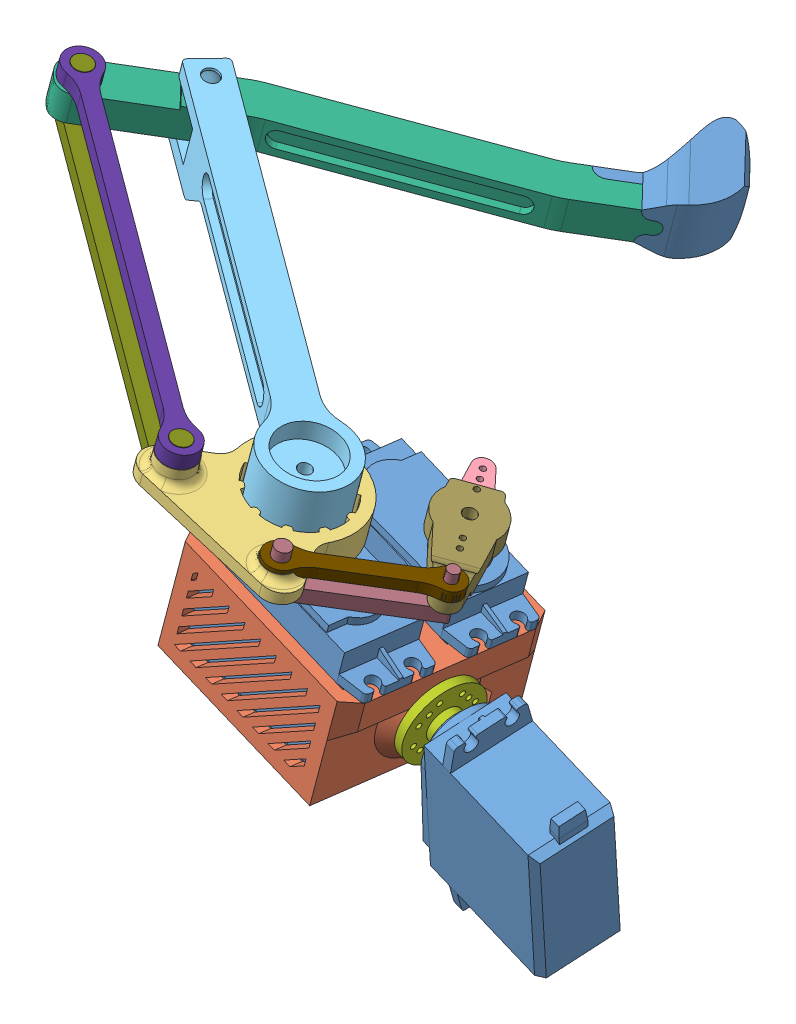
SolidWorks assembly Leg 3, configuration Default. Lengths in mm.
Overall size (184.01 129.02 174.38).
32 component instances, 19 part files, 45 mates.
Components (placement in the parent):
- MG996R-1: MG996R [Default] at (29.5952 -122.5628 58.2658) x (-0.962615 0.249609 -0.105199) z (0.100626 -0.031047 -0.99444) size (54.5 42.75 20)
- MG996R-2: MG996R [Default] at (26.9789 -121.7556 84.1213) x (0.962615 -0.249609 0.105199) z (-0.100626 0.031047 0.99444) size (54.5 42.75 20)
- MG996R-3: MG996R [Default] at (99.0906 -137.4824 76.1232) x (-0.215615 -0.941176 -0.26019) z (0.163956 0.22778 -0.95981) size (54.5 42.75 20)
- Servo Housing-1: Servo Housing [Default] at (37.077 -93.7693 58.1239) x (-0.962615 0.249609 -0.105199) z (0.251487 0.967849 -0.00477) size (61.5 52 29.25)
- Rotating Piece-1: Rotating Piece [Default] at (26.8579 -80.6595 82.9278) x (0.330954 -0.090624 -0.939285) z (0.909518 -0.23464 0.343104) size (44.28 13.7 43.21)
- Double_Blade_Rudder-1: Double_Blade_Rudder [默认] at (51.0424 -81.5852 59.0548) x (0.795547 -0.209518 -0.568514) z (-0.551235 0.13918 -0.82266) size (12.2 5.5 38)
- Upper Leg-1: Upper Leg [Default] at (-58.7777 -49.0599 29.9672) x (-0.525433 0.140664 0.839127) z (0.251487 0.967849 -0.00477) size (22 116.4 18)
- Lower leg-1: Lower leg [Default] at (27.9487 -66.2146 -31.3691) x (0.681118 -0.173478 0.711325) z (-0.251487 -0.967849 0.00477) size (20.21 126 9.59)
- Circle Rudder-1: Circle Rudder [默认] at (57.8128 -116.2822 73.9977) x (0.107242 0.707834 0.698191) z (0.248738 0.660808 -0.70814) size (20.8 5.5 20.8)
- 688ZZ Bearing Assembly-2: 688ZZ Bearing Assembly [Default] at (1.0185 -101.5553 67.791) x (-0.264501 -0.949925 0.166376) z (-0.962615 0.249609 -0.105199) size (17.99 17.98 5)
  - Outer Ring-1: Outer Ring [Default] at origin size (16 16 5)
  - Inner Ring-1: Inner Ring [Default] x (-0.241565 -0.970385 0) z (0 0 1) size (10.6 10.6 5)
  - Cage-1: Cage [Default] x (0.535517 0.844524 0) z (0 0 1) size (13.01 13.06 2.21)
  - 2mm Ball Bearing-1: 2mm Ball Bearing [Default] at (-5.0671 3.2131 0) x (0.050652 0.835774 0.546732) z (0.977207 -0.154478 0.145614) size (2 2 2)
  - 2mm Ball Bearing-2: 2mm Ball Bearing [Default] at (-5.988 -0.3789 0) x (-0.450278 0.705928 0.546732) z (0.881377 0.449412 0.145614) size (2 2 2)
  - 2mm Ball Bearing-3: 2mm Ball Bearing [Default] at (-4.6217 -3.8262 0) x (-0.779216 0.306441 0.546732) z (0.448891 0.881642 0.145614) size (2 2 2)
  - 2mm Ball Bearing-4: 2mm Ball Bearing [Default] at (-1.49 -5.812 0) x (-0.810521 -0.210096 0.546732) z (-0.155056 0.977115 0.145614) size (2 2 2)
  - 2mm Ball Bearing-5: 2mm Ball Bearing [Default] at (2.2108 -5.5778 0) x (-0.532234 -0.646383 0.546732) z (-0.699777 0.699363 0.145614) size (2 2 2)
  - 2mm Ball Bearing-6: 2mm Ball Bearing [Default] at (5.0671 -3.2131 0) x (-0.050652 -0.835774 0.546732) z (-0.977207 0.154478 0.145614) size (2 2 2)
  - 2mm Ball Bearing-7: 2mm Ball Bearing [Default] at (5.988 0.3789 0) x (0.450278 -0.705928 0.546732) z (-0.881377 -0.449412 0.145614) size (2 2 2)
  - 2mm Ball Bearing-8: 2mm Ball Bearing [Default] at (4.6217 3.8262 0) x (0.779216 -0.306441 0.546732) z (-0.448891 -0.881642 0.145614) size (2 2 2)
  - 2mm Ball Bearing-9: 2mm Ball Bearing [Default] at (1.49 5.812 0) x (0.810521 0.210096 0.546732) z (0.155056 -0.977115 0.145614) size (2 2 2)
  - 2mm Ball Bearing-10: 2mm Ball Bearing [Default] at (-2.2108 5.5778 0) x (0.532234 0.646383 0.546732) z (0.699777 -0.699363 0.145614) size (2 2 2)
- Circle Rudder-3: Circle Rudder [默认] at (28.1908 -75.5299 82.9026) x (0.821577 -0.21087 0.529666) z (0.511631 -0.137123 -0.848193) size (20.8 5.5 20.8)
- Servo Arm Mount-1: Servo Arm Mount [Default] at (51.0424 -81.5852 59.0548) x (-0.795547 0.209518 0.568514) z (0.251487 0.967849 -0.00477) size (16.2 34.39 10.1)
- Short Connecting Rod-1: Short Connecting Rod [Default] at (63.2593 -84.1638 75.1548) x (-0.680525 0.180329 0.710188) z (-0.251487 -0.967849 0.00477) size (37.08 6.33 13)
- 91595A167_Dowel Pin-1: 91595A167_Dowel Pin [91595A167] at (-52.4141 -50.7218 28.2719) x (-0.945505 0.244623 -0.214897) z (-0.251487 -0.967849 0.00477) size (4 4 20)
- Rod Cap-2: Rod Cap [Default] at (14.1029 -69.8044 103.5679) x (-0.058992 0.020247 0.998053) z (0.966061 -0.250717 0.062188) size (6.08 7 3)
- Long Connecting Rod-1: Long Connecting Rod [Default] at (14.4682 -71.3647 99.7299) x (0.812824 -0.208525 0.543906) z (-0.251487 -0.967849 0.00477) size (105.4 5 16.7)
- Long Connecting Rod Alt-1: Long Connecting Rod Alt [Default] at (13.1093 -62.8457 100.4303) x (0.812824 -0.208525 0.543906) z (-0.525424 0.140662 0.839132) size (109.5 4 9.1)
- Short Connecting Rod Alt-1: Short Connecting Rod Alt [Default] at (41.5823 -75.0354 101.4606) x (-0.680525 0.180329 0.710188) z (-0.688214 0.175358 -0.703996) size (41.18 3 8.1)
- Foot Cap R2-1: Foot Cap R2 [Default] at (27.9487 -66.2146 -31.3691) x (0.681118 -0.173478 0.711325) z (-0.251487 -0.967849 0.00477) size (26.22 31.5 15)
Mates (geometry in assembly coordinates):
- Coincident3: coincident aligned: plane of MG996R-1 through (49.2065 -88.6505 59.0896) normal (0.251487 0.967849 -0.00477); plane of MG996R-2 through (26.3549 -82.5952 82.9374) normal (0.251487 0.967849 -0.00477)
- Coincident4: coincident aligned: plane of MG996R-1 through (59.0851 -93.3273 50.2812) normal (0.962615 -0.249609 0.105199); plane of MG996R-2 through (54.4563 -91.8991 96.0254) normal (0.962615 -0.249609 0.105199)
- Distance1: distance = 6 mm anti-aligned: plane of MG996R-1 through (57.0726 -92.7063 70.17) normal (-0.100626 0.031047 0.99444); plane of MG996R-2 through (17.4829 -82.4109 71.8761) normal (0.100626 -0.031047 -0.99444)
- InPlace1: in place: plane of ? through (-38.4551 28.1284 17.4765) normal (0 1 0); plane of ? through (0 28.1284 0) normal (0 1 0); moOrthogonalPlaneRef_w of ? through (-38.4551 28.1284 17.4765) normal (0 1 0); plane of ? through (0 28.1284 0) normal (0 0 -1); plane of ? through (-38.4551 28.1284 17.4765) normal (0 1 0); plane of ? through (0 28.1284 0) normal (1 0 0); plane of MG996R-1 through (12.5314 -87.3809 60.2393) normal (0.251487 0.967849 -0.00477); unknown of Servo Housing-1
- Coincident6: coincident aligned: plane of MG996R-1; plane of Servo Housing-1
- Coincident7: coincident aligned: moOrthogonalPlaneRef_w of MG996R-1; plane of Servo Housing-1 through (37.077 -93.7693 58.1239) normal (-0.100626 0.031047 0.99444)
- Coincident8: coincident anti-aligned: moOrthogonalPlaneRef_w of MG996R-1; plane of Servo Housing-1 through (37.077 -93.7693 58.1239) normal (-0.962615 0.249609 -0.105199)
- Concentric4: concentric aligned: cylinder of Upper Leg-1 through (-54.426 -58.4646 28.3101) axis (0.251487 0.967849 -0.00477) radius 2.1; cylinder of Lower leg-1 through (-53.2943 -54.1092 28.2886) axis (0.251487 0.967849 -0.00477) radius 2
- LimitAngle3: limit planar angle = 1.561857 rad anti-aligned: plane of Lower leg-1 through (25.6853 -74.9252 -31.3262) normal (0.681118 -0.173478 0.711325); plane of Upper Leg-1 through (-51.0085 -40.788 21.5283) normal (0.525433 -0.140664 -0.839127)
- Coincident17: coincident anti-aligned: plane of Servo Housing-1 through (36.8825 -202.2704 61.4918) normal (0.962615 -0.249609 0.105199); plane of Circle Rudder-1 through (57.8128 -116.2822 73.9977) normal (-0.962615 0.249609 -0.105199)
- Concentric10: concentric aligned: circle of Servo Housing-1; circle of Circle Rudder-1
- Concentric11: concentric anti-aligned: cylinder of Servo Housing-1 through (-1.388 -100.9312 67.528) axis (0.962615 -0.249609 0.105199) radius 4; cylinder of 688ZZ Bearing Assembly-2/Inner Ring-1 through (-5.4843 -99.8691 67.0803) axis (-0.962615 0.249609 -0.105199) radius 4
- Coincident18: coincident aligned: plane of Servo Housing-1 through (4.1074 -85.2202 54.5209) normal (-0.962615 0.249609 -0.105199); plane of 688ZZ Bearing Assembly-2/Inner Ring-1 through (-2.6372 -105.9123 67.1397) normal (-0.962615 0.249609 -0.105199)
- Coincident19: coincident anti-aligned: plane of MG996R-1 through (50.4639 -83.8113 59.0657) normal (0.251487 0.967849 -0.00477); plane of Circle Rudder-3 through (27.6124 -77.756 82.9135) normal (-0.251487 -0.967849 0.00477)
- Coincident20: coincident anti-aligned: plane of Upper Leg-1 through (28.1908 -75.5299 82.9026) normal (-0.251487 -0.967849 0.00477); plane of Circle Rudder-3 through (28.1908 -75.5299 82.9026) normal (0.251487 0.967849 -0.00477)
- InPlace2: in place: plane of ? through (-72.3336 35.5583 10.554) normal (0 1 0); plane of ? through (0 35.5583 0) normal (0 1 0); plane of ? through (-72.3336 35.5583 10.554) normal (0 1 0); plane of ? through (0 35.5583 0) normal (0 0 -1); plane of ? through (-72.3336 35.5583 10.554) normal (0 1 0); plane of ? through (0 35.5583 0) normal (1 0 0); plane of Double_Blade_Rudder-1 through (51.0424 -81.5852 59.0548) normal (0.251487 0.967849 -0.00477); unknown of Servo Arm Mount-1
- Coincident21: coincident aligned: plane of Double_Blade_Rudder-1; plane of Servo Arm Mount-1
- Coincident22: coincident aligned: moOrthogonalPlaneRef_w of Double_Blade_Rudder-1; plane of Servo Arm Mount-1 through (51.0424 -81.5852 59.0548) normal (0.551235 -0.13918 0.82266)
- Coincident23: coincident anti-aligned: moOrthogonalPlaneRef_w of Double_Blade_Rudder-1; plane of Servo Arm Mount-1 through (51.0424 -81.5852 59.0548) normal (-0.795547 0.209518 0.568514)
- Concentric15: concentric aligned: cylinder of Rotating Piece-1 through (41.5677 -75.0914 101.4609) axis (-0.251487 -0.967849 0.00477) radius 2.2; cylinder of Short Connecting Rod-1 through (43.0263 -69.4779 101.4332) axis (-0.251487 -0.967849 0.00477) radius 2
- Concentric16: concentric anti-aligned: cylinder of Short Connecting Rod-1 through (65.8784 -75.5334 77.5851) axis (-0.251487 -0.967849 0.00477) radius 1.5; cylinder of Servo Arm Mount-1 through (62.4078 -88.8897 77.6509) axis (0.251487 0.967849 -0.00477) radius 1.7
- Concentric18: concentric anti-aligned: cylinder of Upper Leg-1 through (-54.426 -58.4646 28.3101) axis (0.251487 0.967849 -0.00477) radius 2.1; cylinder of 91595A167_Dowel Pin-1 through (-54.9289 -60.4003 28.3196) axis (-0.251487 -0.967849 0.00477) radius 2
- Tangent1: tangent aligned: sphere of 91595A167_Dowel Pin-1; plane of Upper Leg-1 through (-56.2628 -39.3814 29.9195) normal (0.251487 0.967849 -0.00477)
- Concentric24: concentric aligned: cylinder of Circle Rudder-1 through (63.1072 -117.6551 74.5763) axis (-0.962615 0.249609 -0.105199) radius 3; cylinder of MG996R-3 through (63.1072 -117.6551 74.5763) axis (-0.962615 0.249609 -0.105199) radius 1.5
- Concentric28: concentric aligned: cylinder of MG996R-2 through (26.8579 -80.6595 82.9278) axis (0.251487 0.967849 -0.00477) radius 1.5; cylinder of Circle Rudder-3 through (27.6124 -77.756 82.9135) axis (0.251487 0.967849 -0.00477) radius 1.5
- Coincident32: coincident anti-aligned: plane of MG996R-2 through (27.6124 -77.756 82.9135) normal (0.251487 0.967849 -0.00477); plane of Circle Rudder-3 through (27.6124 -77.756 82.9135) normal (-0.251487 -0.967849 0.00477)
- Coincident33: coincident anti-aligned: plane of Upper Leg-1 through (28.1908 -75.5299 82.9026) normal (-0.251487 -0.967849 0.00477); plane of Circle Rudder-3 through (28.1908 -75.5299 82.9026) normal (0.251487 0.967849 -0.00477)
- Concentric29: concentric anti-aligned: cylinder of Upper Leg-1 through (30.4542 -66.8193 82.8596) axis (-0.251487 -0.967849 0.00477) radius 1.7; cylinder of Circle Rudder-3 through (27.6124 -77.756 82.9135) axis (0.251487 0.967849 -0.00477) radius 1.5
- Concentric30: concentric anti-aligned: cylinder of Rotating Piece-1 through (27.3609 -78.7238 82.9183) axis (-0.251487 -0.967849 0.00477) radius 4.35; cylinder of Circle Rudder-3 through (26.8076 -80.8531 82.9288) axis (0.251487 0.967849 -0.00477) radius 4.4
- Coincident34: coincident anti-aligned: plane of MG996R-2 through (26.8579 -80.6595 82.9278) normal (0.251487 0.967849 -0.00477); plane of Rotating Piece-1 through (26.8579 -80.6595 82.9278) normal (-0.251487 -0.967849 0.00477)
- Concentric31: concentric aligned: cylinder of MG996R-1 through (49.7095 -86.7148 59.0801) axis (0.251487 0.967849 -0.00477) radius 1.5; cylinder of Double_Blade_Rudder-1 through (49.6592 -86.9084 59.081) axis (0.251487 0.967849 -0.00477) radius 3
- Coincident35: coincident anti-aligned: plane of MG996R-1 through (50.4639 -83.8113 59.0657) normal (0.251487 0.967849 -0.00477); plane of Double_Blade_Rudder-1 through (50.4639 -83.8113 59.0657) normal (-0.251487 -0.967849 0.00477)
- Coincident36: coincident anti-aligned: plane of MG996R-3 through (63.1072 -117.6551 74.5763) normal (-0.962615 0.249609 -0.105199); plane of Circle Rudder-1 through (63.1072 -117.6551 74.5763) normal (0.962615 -0.249609 0.105199)
- Coincident37: coincident anti-aligned: plane of Servo Arm Mount-1 through (63.615 -84.244 77.6281) normal (-0.251487 -0.967849 0.00477); plane of Short Connecting Rod-1 through (100.6566 -93.5641 139.4827) normal (0.251487 0.967849 -0.00477)
- Concentric32: concentric anti-aligned: cylinder of Rotating Piece-1 through (11.9274 -67.3946 100.4527) axis (-0.251487 -0.967849 0.00477) radius 2.7; cylinder of Long Connecting Rod-1 through (10.1166 -74.3631 100.4871) axis (0.251487 0.967849 -0.00477) radius 2.5
- Concentric33: concentric aligned: cylinder of Lower leg-1 through (-70.485 -49.5558 45.8598) axis (0.251487 0.967849 -0.00477) radius 2.6; cylinder of Long Connecting Rod-1 through (-71.4909 -53.4272 45.8789) axis (0.251487 0.967849 -0.00477) radius 2.5
- Coincident38: coincident anti-aligned: plane of Lower leg-1 through (25.6853 -74.9252 -31.3262) normal (-0.251487 -0.967849 0.00477); plane of Long Connecting Rod-1 through (14.4682 -71.3647 99.7299) normal (0.251487 0.967849 -0.00477)
- Concentric34: concentric anti-aligned: cylinder of Long Connecting Rod-1 through (-71.4909 -53.4272 45.8789) axis (0.251487 0.967849 -0.00477) radius 2.5; cylinder of Long Connecting Rod Alt-1 through (-67.4923 -38.0384 45.803) axis (-0.251487 -0.967849 0.00477) radius 2.55
- Distance2: distance = 0.5 mm anti-aligned: plane of Lower leg-1 through (27.9487 -66.2146 -31.3691) normal (0.251487 0.967849 -0.00477); plane of Upper Leg-1 through (-48.8618 -45.5034 16.5126) normal (-0.251487 -0.967849 0.00477)
- Coincident40: coincident anti-aligned: plane of Rotating Piece-1 through (13.1093 -62.8457 100.4303) normal (0.251487 0.967849 -0.00477); plane of Long Connecting Rod Alt-1 through (13.1093 -62.8457 100.4303) normal (-0.251487 -0.967849 0.00477)
- Concentric35: concentric anti-aligned: cylinder of Long Connecting Rod-1 through (10.1166 -74.3631 100.4871) axis (0.251487 0.967849 -0.00477) radius 2.5; cylinder of Long Connecting Rod Alt-1 through (14.1153 -58.9743 100.4112) axis (-0.251487 -0.967849 0.00477) radius 2.55
- Concentric36: concentric aligned: cylinder of Short Connecting Rod-1 through (65.8784 -75.5334 77.5851) axis (-0.251487 -0.967849 0.00477) radius 1.5; cylinder of Short Connecting Rod Alt-1 through (65.1888 -78.1873 77.5982) axis (-0.251487 -0.967849 0.00477) radius 1.55
- Concentric37: concentric aligned: cylinder of Short Connecting Rod-1 through (43.0263 -69.4779 101.4332) axis (-0.251487 -0.967849 0.00477) radius 2; cylinder of Short Connecting Rod Alt-1 through (42.3367 -72.1318 101.4463) axis (-0.251487 -0.967849 0.00477) radius 2.05
- Concentric38: concentric aligned: cylinder of Lower leg-1 through (8.6274 -65.7865 -19.7931) axis (-0.681118 0.173478 -0.711325) radius 2; cylinder of Foot Cap R2-1 through (8.6274 -65.7865 -19.7931) axis (-0.681118 0.173478 -0.711325) radius 2
- Concentric39: concentric aligned: cylinder of Lower leg-1 through (20.4173 -64.2543 -30.7087) axis (-0.251487 -0.967849 0.00477) radius 2; cylinder of Foot Cap R2-1 through (20.4173 -64.2543 -30.7087) axis (-0.251487 -0.967849 0.00477) radius 2
